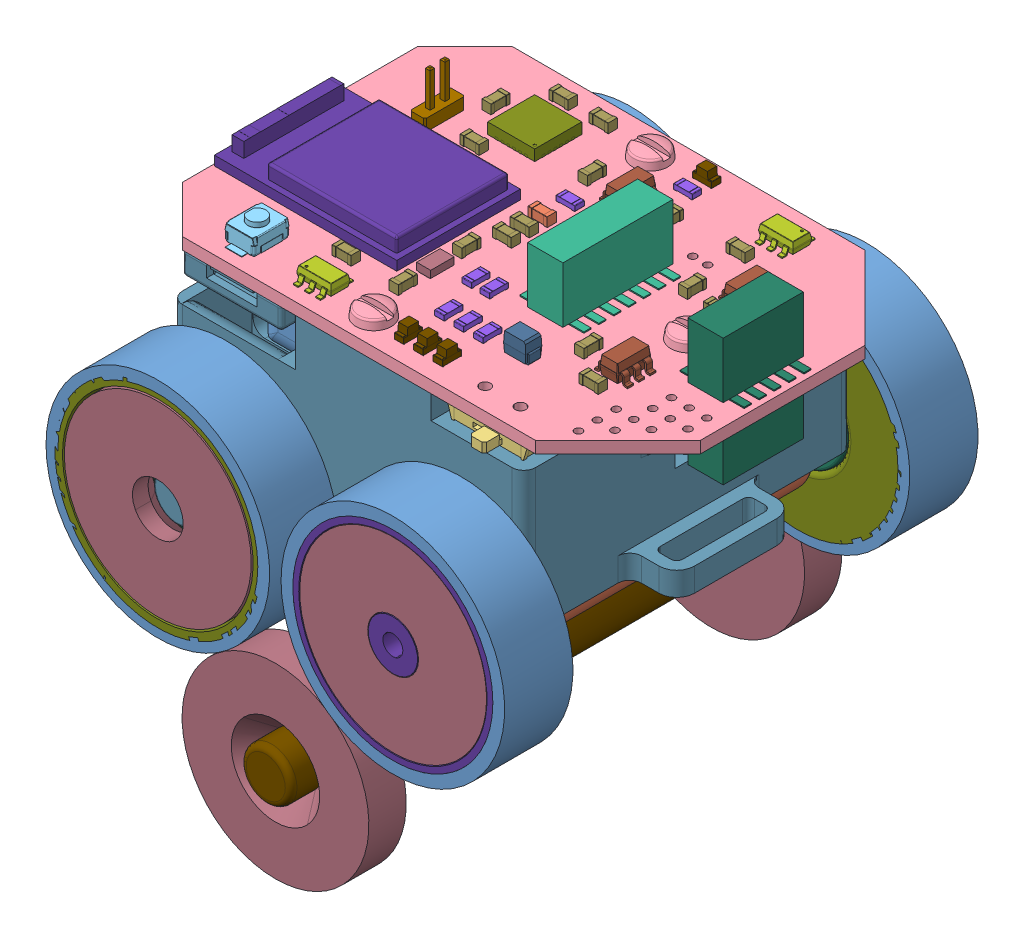
SolidWorks assembly AstroAnt, configuration Default. Lengths in mm.
Overall size (43.74 45.41 41.85).
158 component instances, 38 part files, 43 mates.
Components (placement in the parent):
- LiPo_360mAh-1: LiPo_360mAh [Default] at (6.8166 4.9998 44.2756) size (25 7 18)
- PA2-50-1: PA2-50 [Default] at (8.0673 -18.301 41.8029) x (0 0 1) z (0.952879 0.303349 0) size (29.1 8 8)
- PA2-50-2: PA2-50 [Default] at (-4.1563 19.5334 49.6029) x (0 0 -1) z (0.755989 -0.654584 0) size (29.1 8 8)
- 92120A150_Brass Heat-Set Inserts for Plastic-1: 92120A150_Brass Heat-Set Inserts for Plastic [92120A150] at (19.9543 12.4998 45.7029) size (2.56 3.33 2.56)
- 92120A150_Brass Heat-Set Inserts for Plastic-2: 92120A150_Brass Heat-Set Inserts for Plastic [92120A150] at (4.9543 12.4998 33.9529) size (2.56 3.33 2.56)
- 92120A150_Brass Heat-Set Inserts for Plastic-3: 92120A150_Brass Heat-Set Inserts for Plastic [92120A150] at (4.9543 12.4998 57.4529) size (2.56 3.33 2.56)
- 91460A005_METRIC CHEESE HEAD SLOTTED MACHINE SCREW-8: 91460A005_METRIC CHEESE HEAD SLOTTED MACHINE SCREW [91460A005] at (4.9543 14.9998 57.4529) x (1 0 0) z (0 1 0) size (3 3 7.1)
- 91460A005_METRIC CHEESE HEAD SLOTTED MACHINE SCREW-9: 91460A005_METRIC CHEESE HEAD SLOTTED MACHINE SCREW [91460A005] at (4.9543 14.9998 33.9529) x (1 0 0) z (0 1 0) size (3 3 7.1)
- 91460A005_METRIC CHEESE HEAD SLOTTED MACHINE SCREW-10: 91460A005_METRIC CHEESE HEAD SLOTTED MACHINE SCREW [91460A005] at (19.9543 14.9998 45.7029) x (1 0 0) z (0 1 0) size (3 3 7.1)
- 92120A150_Brass Heat-Set Inserts for Plastic-4: 92120A150_Brass Heat-Set Inserts for Plastic [92120A150] at (4.9543 1.4998 57.4529) x (-0.616962 0 -0.786993) z (0.786993 0 -0.616962) size (2.56 3.33 2.56)
- 92120A150_Brass Heat-Set Inserts for Plastic-5: 92120A150_Brass Heat-Set Inserts for Plastic [92120A150] at (4.9543 1.4998 33.9529) x (-0.616962 0 -0.786993) z (0.786993 0 -0.616962) size (2.56 3.33 2.56)
- 91460A005_METRIC CHEESE HEAD SLOTTED MACHINE SCREW-14: 91460A005_METRIC CHEESE HEAD SLOTTED MACHINE SCREW [91460A005] at (4.9543 -2.5002 57.4529) x (0.663599 0 0.748089) z (0 -1 0) size (3 3 7.1)
- 91460A005_METRIC CHEESE HEAD SLOTTED MACHINE SCREW-15: 91460A005_METRIC CHEESE HEAD SLOTTED MACHINE SCREW [91460A005] at (4.9543 -2.5002 33.9529) x (0.663599 0 0.748089) z (0 -1 0) size (3 3 7.1)
- mainboard_v1.step-1: mainboard_v1.step [Default] at (-103.0457 13.9998 235.7029) x (0 0 -1) z (0 1 0) size (29.41 41 10.8)
  - B3U-1000P.step-1: B3U-1000P.step [Default] at (178.95 -97.38 1.05) x (1 0 0) z (0 -1 0) size (4 1.75 2.5)
    - COMPOUND.step-1: COMPOUND.step [Default] at origin size (4 1.75 2.5)
  - 20021321-00014C1LF.step-1: 20021321-00014C1LF.step [Default] at (190 -115.5 1.05) size (9.35 5.45 4.85)
    - COMPOUND-0.step-1: COMPOUND-0.step [Default] at origin size (9.35 5.45 4.85)
  - MP6513GJ-Z.step-1: MP6513GJ-Z.step [Default] at (201.21 -120 1.05) x (-1 0 0) z (0 0 1) size (2.8 2.9 1)
    - COMPOUND-1.step-1: COMPOUND-1.step [Default] at origin size (2.8 2.9 1)
  - MP6513GJ-Z.step-2: MP6513GJ-Z.step [Default] at (178.51 -103.46 1.05) size (2.8 2.9 1)
    - COMPOUND-1.step-1: COMPOUND-1.step [Default] at origin size (2.8 2.9 1)
  - R_0603_1608Metric.step-1: R_0603_1608Metric.step [Default] at (195.55 -104.38 -0.05) x (1 0 0) z (0 0 -1) size (1.6 0.8 0.45)
    - SOLID.step-1: SOLID.step [Default] at origin size (1.6 0.8 0.45)
  - R_0603_1608Metric.step-2: R_0603_1608Metric.step [Default] at (192.6 -99.86 -0.05) x (0 1 0) z (0 0 -1) size (1.6 0.8 0.45)
    - SOLID.step-1: SOLID.step [Default] at origin size (1.6 0.8 0.45)
  - PinHeader_2x01_P1.27mm_Vertical.step-1: PinHeader_2x01_P1.27mm_Vertical.step [Default] at (194.96 -96.07 1.05) size (3.4 1.27 6.3)
    - SOLID-2.step-1: SOLID-2.step [Default] at origin size (3.4 1.27 6.3)
  - TAJP106K010RNJ.step-1: TAJP106K010RNJ.step [Default] at (196.22 -98.14 -0.05) x (-1 0 0) z (0 0 -1) size (2.05 1.4 1.7)
    - COMPOUND-3.step-1: COMPOUND-3.step [Default] at origin size (2.05 1.4 1.7)
  - TAJP106K010RNJ.step-2: TAJP106K010RNJ.step [Default] at (181.68 -117.23 1.05) x (0 1 0) z (0 0 1) size (2.05 1.4 1.7)
    - COMPOUND-3.step-1: COMPOUND-3.step [Default] at origin size (2.05 1.4 1.7)
  - SOT-23-5.step-1: SOT-23-5.step [Default] at (195.38 -122.78 1.05) x (0 1 0) z (0 0 1) size (2.8 2.9 1.55)
    - SOLID-4.step-1: SOLID-4.step [Default] at origin size (2.8 2.9 1.55)
  - C_0603_1608Metric.step-1: C_0603_1608Metric.step [Default] at (192.91 -122.55 1.05) x (0 -1 0) z (0 0 1) size (1.6 0.8 0.8)
    - SOLID-5.step-1: SOLID-5.step [Default] at origin size (1.6 0.8 0.8)
  - C_0603_1608Metric.step-2: C_0603_1608Metric.step [Default] at (193.57 -119.76 1.05) size (1.6 0.8 0.8)
    - SOLID-5.step-1: SOLID-5.step [Default] at origin size (1.6 0.8 0.8)
  - ECS-.327-12.5-12-TR.step-1: ECS-.327-12.5-12-TR.step [Default] at (184.31 -107.18 1.05) size (2 1.2 0.7)
    - COMPOUND-6.step-1: COMPOUND-6.step [Default] at origin size (2 1.2 0.7)
  - C_0603_1608Metric.step-3: C_0603_1608Metric.step [Default] at (197.67 -113.69 1.05) size (1.6 0.8 0.8)
    - SOLID-5.step-1: SOLID-5.step [Default] at origin size (1.6 0.8 0.8)
  - C_0603_1608Metric.step-4: C_0603_1608Metric.step [Default] at (197.64 -107.18 1.05) size (1.6 0.8 0.8)
    - SOLID-5.step-1: SOLID-5.step [Default] at origin size (1.6 0.8 0.8)
  - C_0603_1608Metric.step-5: C_0603_1608Metric.step [Default] at (190.96 -108.09 1.05) x (0 1 0) z (0 0 1) size (1.6 0.8 0.8)
    - SOLID-5.step-1: SOLID-5.step [Default] at origin size (1.6 0.8 0.8)
  - 1734592-6.step-1: 1734592-6.step [Default] at (203.79 -118 -1.05) x (0 -1 0) z (1 0 0) size (8.43 2.05 5.11)
    - SOLID-7.step-1: SOLID-7.step [Default] at origin size (8.43 2.05 5.11)
  - 1734592-6.step-2: 1734592-6.step [Default] at (176.19 -98 -1.05) x (0 1 0) z (-1 0 0) size (8.43 2.05 5.11)
    - SOLID-7.step-1: SOLID-7.step [Default] at origin size (8.43 2.05 5.11)
  - 20021321-00010C4LF.step-1: 20021321-00010C4LF.step [Default] at (190 -127.85 -0.05) x (1 0 0) z (0 0 -1) size (6.81 5.45 4.85)
    - COMPOUND-8.step-1: COMPOUND-8.step [Default] at origin size (6.81 5.45 4.85)
  - 20021321-00010C4LF.step-2: 20021321-00010C4LF.step [Default] at (190 -127.85 1.05) size (6.81 5.45 4.85)
    - COMPOUND-8.step-1: COMPOUND-8.step [Default] at origin size (6.81 5.45 4.85)
  - C_0603_1608Metric.step-6: C_0603_1608Metric.step [Default] at (181.31 -102.6 1.05) x (0 -1 0) z (0 0 1) size (1.6 0.8 0.8)
    - SOLID-5.step-1: SOLID-5.step [Default] at origin size (1.6 0.8 0.8)
  - C_0603_1608Metric.step-7: C_0603_1608Metric.step [Default] at (198.25 -119.14 1.05) x (0 -1 0) z (0 0 1) size (1.6 0.8 0.8)
    - SOLID-5.step-1: SOLID-5.step [Default] at origin size (1.6 0.8 0.8)
  - MPU6050.step-1: MPU6050.step [Default] at (198.43 -101.5 1.05) x (0 1 0) z (1 0 0) size (4 0.95 4)
    - COMPOUND-9.step-1: COMPOUND-9.step [Default] at origin size (4 0.95 4)
  - C_0603_1608Metric.step-8: C_0603_1608Metric.step [Default] at (194.9 -99.89 1.05) x (0 -1 0) z (0 0 1) size (1.6 0.8 0.8)
    - SOLID-5.step-1: SOLID-5.step [Default] at origin size (1.6 0.8 0.8)
  - C_0603_1608Metric.step-9: C_0603_1608Metric.step [Default] at (201.98 -100.38 1.05) x (0 -1 0) z (0 0 1) size (1.6 0.8 0.8)
    - SOLID-5.step-1: SOLID-5.step [Default] at origin size (1.6 0.8 0.8)
  - C_0603_1608Metric.step-10: C_0603_1608Metric.step [Default] at (201.98 -103.78 1.05) x (0 1 0) z (0 0 1) size (1.6 0.8 0.8)
    - SOLID-5.step-1: SOLID-5.step [Default] at origin size (1.6 0.8 0.8)
  - C_0603_1608Metric.step-11: C_0603_1608Metric.step [Default] at (198.81 -97.82 1.05) size (1.6 0.8 0.8)
    - SOLID-5.step-1: SOLID-5.step [Default] at origin size (1.6 0.8 0.8)
  - SOT-23-5.step-2: SOT-23-5.step [Default] at (184.86 -122.77 1.05) x (0 1 0) z (0 0 1) size (2.8 2.9 1.55)
    - SOLID-4.step-1: SOLID-4.step [Default] at origin size (2.8 2.9 1.55)
  - SOT-23-5.step-3: SOT-23-5.step [Default] at (197.58 -110.46 1.05) x (0 1 0) z (0 0 1) size (2.8 2.9 1.55)
    - SOLID-4.step-1: SOLID-4.step [Default] at origin size (2.8 2.9 1.55)
  - MDBT50Q-1MV2.step-1: MDBT50Q-1MV2.step [Default] at (187.3136 -98.605 1.0754) x (-1 0 0) z (0 1 0) size (10.5 2.06 15.5)
    - SOLID-10.step-1: SOLID-10.step [Default] at origin size (10.5 2.06 15.5)
  - C_0603_1608Metric.step-12: C_0603_1608Metric.step [Default] at (189.44 -108.09 1.05) x (0 1 0) z (0 0 1) size (1.6 0.8 0.8)
    - SOLID-5.step-1: SOLID-5.step [Default] at origin size (1.6 0.8 0.8)
  - C_0603_1608Metric.step-13: C_0603_1608Metric.step [Default] at (181.57 -107.18 1.05) x (-1 0 0) z (0 0 1) size (1.6 0.8 0.8)
    - SOLID-5.step-1: SOLID-5.step [Default] at origin size (1.6 0.8 0.8)
  - C_0603_1608Metric.step-14: C_0603_1608Metric.step [Default] at (186.97 -107.18 1.05) size (1.6 0.8 0.8)
    - SOLID-5.step-1: SOLID-5.step [Default] at origin size (1.6 0.8 0.8)
  - C_0603_1608Metric.step-15: C_0603_1608Metric.step [Default] at (184.77 -119.75 1.05) x (-1 0 0) z (0 0 1) size (1.6 0.8 0.8)
    - SOLID-5.step-1: SOLID-5.step [Default] at origin size (1.6 0.8 0.8)
  - C_0603_1608Metric.step-16: C_0603_1608Metric.step [Default] at (182.37 -122.54 1.05) x (0 -1 0) z (0 0 1) size (1.6 0.8 0.8)
    - SOLID-5.step-1: SOLID-5.step [Default] at origin size (1.6 0.8 0.8)
  - LED_0603_1608Metric.step-1: LED_0603_1608Metric.step [Default] at (178.19 -111.01 1.05) size (1.6 0.8 1.1)
    - SOLID-11.step-1: SOLID-11.step [Default] at origin size (1.6 0.8 1.1)
  - LED_0603_1608Metric.step-2: LED_0603_1608Metric.step [Default] at (178.19 -112.66 1.05) size (1.6 0.8 1.1)
    - SOLID-11.step-1: SOLID-11.step [Default] at origin size (1.6 0.8 1.1)
  - LED_0603_1608Metric.step-3: LED_0603_1608Metric.step [Default] at (178.19 -114.31 1.05) size (1.6 0.8 1.1)
    - SOLID-11.step-1: SOLID-11.step [Default] at origin size (1.6 0.8 1.1)
  - LED_0603_1608Metric.step-4: LED_0603_1608Metric.step [Default] at (202.34 -112.21 1.05) x (0 1 0) z (0 0 1) size (1.6 0.8 1.1)
    - SOLID-11.step-1: SOLID-11.step [Default] at origin size (1.6 0.8 1.1)
  - 473460001.step-1: 473460001.step [Default] at (201.68 -99.72 -1.25) x (0 -1 0) z (1 0 0) size (7.98 2.94 5.43)
    - COMPOUND-12.step-1: COMPOUND-12.step [Default] at origin size (7.98 2.94 5.43)
  - L_0603_1608Metric.step-1: L_0603_1608Metric.step [Default] at (192.48 -108.09 1.05) x (0 1 0) z (0 0 1) size (1.6 0.8 0.8)
    - SOLID-13.step-1: SOLID-13.step [Default] at origin size (1.6 0.8 0.8)
  - R_0603_1608Metric.step-3: R_0603_1608Metric.step [Default] at (185.18 -111.31 1.05) x (-1 0 0) z (0 0 1) size (1.6 0.8 0.45)
    - SOLID.step-1: SOLID.step [Default] at origin size (1.6 0.8 0.45)
  - R_0603_1608Metric.step-4: R_0603_1608Metric.step [Default] at (185.18 -109.77 1.05) size (1.6 0.8 0.45)
    - SOLID.step-1: SOLID.step [Default] at origin size (1.6 0.8 0.45)
  - R_0603_1608Metric.step-5: R_0603_1608Metric.step [Default] at (181.62 -111.01 1.05) size (1.6 0.8 0.45)
    - SOLID.step-1: SOLID.step [Default] at origin size (1.6 0.8 0.45)
  - R_0603_1608Metric.step-6: R_0603_1608Metric.step [Default] at (181.62 -112.66 1.05) size (1.6 0.8 0.45)
    - SOLID.step-1: SOLID.step [Default] at origin size (1.6 0.8 0.45)
  - R_0603_1608Metric.step-7: R_0603_1608Metric.step [Default] at (181.62 -114.31 1.05) x (-1 0 0) z (0 0 1) size (1.6 0.8 0.45)
    - SOLID.step-1: SOLID.step [Default] at origin size (1.6 0.8 0.45)
  - R_0603_1608Metric.step-8: R_0603_1608Metric.step [Default] at (194.84 -108.1 1.05) x (0 1 0) z (0 0 1) size (1.6 0.8 0.45)
    - SOLID.step-1: SOLID.step [Default] at origin size (1.6 0.8 0.45)
  - R_0603_1608Metric.step-9: R_0603_1608Metric.step [Default] at (200.69 -112.2325 1.05) x (0 1 0) z (0 0 1) size (1.6 0.8 0.45)
    - SOLID.step-1: SOLID.step [Default] at origin size (1.6 0.8 0.45)
  - R_0603_1608Metric.step-10: R_0603_1608Metric.step [Default] at (196.22 -101.51 -0.05) x (-1 0 0) z (0 0 -1) size (1.6 0.8 0.45)
    - SOLID.step-1: SOLID.step [Default] at origin size (1.6 0.8 0.45)
  - R_0603_1608Metric.step-11: R_0603_1608Metric.step [Default] at (196.22 -99.9725 -0.05) x (-1 0 0) z (0 0 -1) size (1.6 0.8 0.45)
    - SOLID.step-1: SOLID.step [Default] at origin size (1.6 0.8 0.45)
  - SW_SPDT_PCM12.step-1: SW_SPDT_PCM12.step [Default] at (178.18 -119.37 -0.05) x (0 1 0) z (0 0 -1) size (7.7 5 2)
    - SOLID-14.step-1: SOLID-14.step [Default] at origin size (7.7 5 2)
  - COMPOUND-15.step-1: COMPOUND-15.step [Default] at origin size (28 41 1)
- 91613A020_METRIC CHEESE HEAD SLOTTED MACHINE SCREW-1: 91613A020_METRIC CHEESE HEAD SLOTTED MACHINE SCREW [91613A020] at (1.2533 -0.5002 54.4029) x (1 0 0) z (0 1 0) size (3 3 5.08)
- 91613A020_METRIC CHEESE HEAD SLOTTED MACHINE SCREW-2: 91613A020_METRIC CHEESE HEAD SLOTTED MACHINE SCREW [91613A020] at (8.6533 -0.5002 54.4029) x (1 0 0) z (0 1 0) size (3 3 5.08)
- 91613A020_METRIC CHEESE HEAD SLOTTED MACHINE SCREW-3: 91613A020_METRIC CHEESE HEAD SLOTTED MACHINE SCREW [91613A020] at (1.2533 -0.5002 37.0029) x (1 0 0) z (0 1 0) size (3 3 5.08)
- IR_TEMP_V2.step-3: IR_TEMP_V2.step [Default] at (118.9553 -0.5002 109.7029) x (-1 0 0) z (0 1 0) size (10 20 4.8)
  - Board_Geoms_380f.step-1: Board_Geoms_380f.step [Default] at origin size (10 20 1.11)
    - Pcb_380f.step-1: Pcb_380f.step [Default] at origin size (10 20 1)
    - topTracks_380f.step-1: topTracks_380f.step [Default] at (0 0 0.01) size (9.62 17.53 0.05)
    - botTracks_380f.step-1: botTracks_380f.step [Default] at (0 0 -1.01) size (9.25 16.88 0.05)
  - Step_Models_380f.step-1: Step_Models_380f.step [Default] at origin size (9.46 10.17 4.8)
    - Top_380f.step-1: Top_380f.step [Default] at origin size (9.46 10.17 1.2)
      - IC1_PW14_613E6C6D.step-1: IC1_PW14_613E6C6D.step [Default] at (113.99 -59.48 0) x (-1 0 0) z (0 1 0) size (6.4 1.2 5)
      - C1_C_0402_1005Metric_613EDDF6.step-1: C1_C_0402_1005Metric_613EDDF6.step [Default] at (110.5 -64.26 0) x (-1 0 0) z (0 0 1) size (1 0.5 0.5)
      - C1_C_0402_1005Metric_613EDDF6.step-2: C1_C_0402_1005Metric_613EDDF6.step [Default] at (109.52 -61.07 0) x (0 -1 0) z (0 0 1) size (1 0.5 0.5)
      - C1_C_0402_1005Metric_613EDDF6.step-3: C1_C_0402_1005Metric_613EDDF6.step [Default] at (118.48 -60.86 0) x (0 -1 0) z (0 0 1) size (1 0.5 0.5)
      - C1_C_0402_1005Metric_613EDDF6.step-4: C1_C_0402_1005Metric_613EDDF6.step [Default] at (118.48 -58.59 0) x (0 -1 0) z (0 0 1) size (1 0.5 0.5)
      - C1_C_0402_1005Metric_613EDDF6.step-5: C1_C_0402_1005Metric_613EDDF6.step [Default] at (113.32 -66.9 0) size (1 0.5 0.5)
      - R1_R_0402_1005Metric_613EDE7A.step-1: R1_R_0402_1005Metric_613EDE7A.step [Default] at (110.98 -63.1 0) size (1 0.5 0.35)
      - R1_R_0402_1005Metric_613EDE7A.step-2: R1_R_0402_1005Metric_613EDE7A.step [Default] at (111.68 -66.3 0) x (0 1 0) z (0 0 1) size (1 0.5 0.35)
    - Bot_380f.step-1: Bot_380f.step [Default] at origin size (6.35 7.64 4.6)
      - U1_ZTP-135SR_613E6CD4.step-1: U1_ZTP-135SR_613E6CD4.step [Default] at (114 -64 -1) x (-1 0 0) z (0 -1 0) size (6.35 4.6 5.4)
      - C1_C_0402_1005Metric_613EDDF6.step-1: C1_C_0402_1005Metric_613EDDF6.step [Default] at (115.07 -59.56 -1) x (0 -1 0) z (0 0 -1) size (1 0.5 0.5)
      - R1_R_0402_1005Metric_613EDE7A.step-1: R1_R_0402_1005Metric_613EDE7A.step [Default] at (113.64 -59.58 -1) x (0 -1 0) z (0 0 -1) size (1 0.5 0.35)
- RA22CS-N.step-3: RA22CS-N.step [Default] at (-5.0457 -0.0002 27.1904) x (0.93329 0.359123 0) z (0.359123 -0.93329 0) size (15.88 3.17 15.88)
- Body_simple-1: Body_simple [Default] at (4.8007 -0.0002 38.7677) size (34 16 37)
- RA22CS-N.step-4: RA22CS-N.step [Default] at (14.9543 -0.0002 27.1904) x (0.986453 0.164042 0) z (0.164042 -0.986453 0) size (15.88 3.17 15.88)
- RA22CS-N.step-5: RA22CS-N.step [Default] at (4.9543 -14.2854 27.1904) x (0.988519 -0.1511 0) z (0.1511 0.988519 0) size (15.88 3.17 15.88)
- ball_bearing_5x11x4mm-1: ball_bearing_5x11x4mm [Default] at (-45.4624 -2.1758 28.9029) x (0.999925 -0.012245 0) z (0 0 1) size (8 8 2.5)
- wheel_holder_non_motor-1: wheel_holder_non_motor [Default] at (-70.2522 1.7638 25.6029) size (17.5 17.5 5.8)
- wheel_holder_non_motor-2: wheel_holder_non_motor [Default] at (-19.1131 -84.0559 65.8029) x (0.185441 0.982655 0) z (0 0 -1) size (17.5 17.5 5.8)
- ball_bearing_5x11x4mm-2: ball_bearing_5x11x4mm [Default] at (-30.2803 -54.9376 62.5029) x (0.373101 0.927791 0) z (0 0 -1) size (8 8 2.5)
- RA22CS-N.step-6: RA22CS-N.step [Default] at (-5.0457 -0.0002 64.2154) x (-0.469735 0.882807 0) z (-0.882807 -0.469735 0) size (15.88 3.17 15.88)
- RA22CS-N.step-7: RA22CS-N.step [Default] at (14.9543 -0.0002 64.2154) x (-0.206529 0.978441 0) z (-0.978441 -0.206529 0) size (15.88 3.17 15.88)
- wheel_motor-1: wheel_motor [Default] at (24.0366 1.7037 25.5779) size (17 17 5.8)
- wheel_motor-2: wheel_motor [Default] at (15.5431 29.126 65.8279) x (-0.038296 0.999266 0) z (0 0 -1) size (17 17 5.8)
- RA22CS-N.step-8: RA22CS-N.step [Default] at (4.9543 -14.2854 64.2154) x (-0.693236 -0.720711 0) z (-0.720711 0.693236 0) size (15.88 3.17 15.88)
- magnet_wheel_holder-1: magnet_wheel_holder [Default] at (28.927 -0.7064 28.7779) size (6 6 41.85)
- tire-1: tire [Default] at (38.167 -1.442 25.5779) size (19 19 5.8)
- tire-2: tire [Default] at (58.167 -1.442 25.6029) size (19 19 5.8)
- tire-3: tire [Default] at (38.167 -1.442 60.0029) size (19 19 5.8)
- tire-4: tire [Default] at (58.167 -1.442 60.0279) size (19 19 5.8)
- motor_holder-2: motor_holder [Default] at (-0.192 -4.5002 11.9282) size (20 4.13 28)
Mates (geometry in assembly coordinates):
- Coincident100: coincident anti-aligned: plane of mainboard_v1.step-1/COMPOUND-15.step-1 through (6.7692 13.9998 45.7029) normal (0 -1 0); plane of Body_simple-1 through (4.8007 13.9998 38.7677) normal (0 1 0)
- Concentric58: concentric anti-aligned: cylinder of PA2-50-2 through (-5.0457 -0.0002 33.4029) axis (0 0 1) radius 4; cylinder of Body_simple-1 through (-5.0457 -0.0002 57.7029) axis (0 0 -1) radius 4.1
- Concentric59: concentric aligned: cylinder of mainboard_v1.step-1/COMPOUND-15.step-1 through (19.9543 13.4998 45.7029) axis (0 1 0) radius 0.85; cylinder of Body_simple-1 through (19.9543 5.9998 45.7029) axis (0 1 0) radius 1.15
- Concentric60: concentric anti-aligned: cylinder of PA2-50-2 through (-5.0457 -0.0002 29.3029) axis (0 0 1) radius 1; cylinder of RA22CS-N.step-3 through (-5.0457 -0.0002 27.1904) axis (0 0 -1) radius 2.159
- Concentric63: concentric anti-aligned: cylinder of ball_bearing_5x11x4mm-1 through (14.9543 -0.0002 31.4029) axis (0 0 -1) radius 4; cylinder of wheel_holder_non_motor-1 through (14.9543 -0.0002 25.6029) axis (0 0 1) radius 4
- Concentric64: concentric aligned: cylinder of RA22CS-N.step-4 through (14.9543 -0.0002 28.7779) axis (0 0 -1) radius 7.9375; cylinder of wheel_holder_non_motor-1 through (14.9543 -0.0002 28.8029) axis (0 0 -1) radius 8.1
- Coincident103: coincident aligned: plane of RA22CS-N.step-4 through (14.9543 -0.0002 25.6029) normal (0 0 -1); plane of wheel_holder_non_motor-1 through (14.9543 -0.0002 25.6029) normal (0 0 -1)
- Concentric66: concentric anti-aligned: cylinder of Body_simple-1 through (14.9543 -0.0002 27.2029) axis (0 0 1) radius 2; cylinder of ball_bearing_5x11x4mm-1 through (14.9543 -0.0002 32.9029) axis (0 0 -1) radius 2
- Distance2: distance = 0.3 mm anti-aligned: plane of wheel_holder_non_motor-1 through (14.9543 -0.0002 31.4029) normal (0 0 1); plane of Body_simple-1 through (-10.0457 13.9998 31.7029) normal (0 0 -1)
- Coincident105: coincident aligned: plane of ball_bearing_5x11x4mm-1 through (14.9543 -0.0002 31.4029) normal (0 0 1); plane of wheel_holder_non_motor-1 through (14.9543 -0.0002 31.4029) normal (0 0 1)
- Distance3: distance = 0.3 mm anti-aligned: plane of wheel_holder_non_motor-2 through (-5.0457 -0.0002 60.0029) normal (0 0 -1); plane of Body_simple-1 through (-10.0457 13.9998 59.7029) normal (0 0 1)
- Concentric67: concentric aligned: cylinder of Body_simple-1 through (-5.0457 -0.0002 64.2029) axis (0 0 -1) radius 2; cylinder of wheel_holder_non_motor-2 through (-5.0457 -0.0002 65.8029) axis (0 0 -1) radius 4
- Coincident107: coincident aligned: plane of wheel_holder_non_motor-2 through (-5.0457 -0.0002 60.0029) normal (0 0 -1); plane of ball_bearing_5x11x4mm-2 through (-5.0457 -0.0002 60.0029) normal (0 0 -1)
- Concentric68: concentric anti-aligned: cylinder of Body_simple-1 through (-5.0457 -0.0002 64.2029) axis (0 0 -1) radius 2; cylinder of ball_bearing_5x11x4mm-2 through (-5.0457 -0.0002 58.5029) axis (0 0 1) radius 2
- Concentric69: concentric anti-aligned: cylinder of Body_simple-1 through (-5.0457 -0.0002 64.2029) axis (0 0 -1) radius 2; cylinder of RA22CS-N.step-6 through (-5.0457 -0.0002 64.2154) axis (0 0 1) radius 2.159
- Coincident108: coincident aligned: plane of wheel_holder_non_motor-2 through (-5.0457 -0.0002 65.8029) normal (0 0 1); plane of RA22CS-N.step-6 through (-5.0457 -0.0002 65.8029) normal (0 0 1)
- Coincident109: coincident aligned: plane of RA22CS-N.step-3 through (-5.0457 -0.0002 25.6029) normal (0 0 -1); plane of RA22CS-N.step-4 through (14.9543 -0.0002 25.6029) normal (0 0 -1)
- Concentric70: concentric anti-aligned: cylinder of PA2-50-2 through (-5.0457 -0.0002 29.3029) axis (0 0 1) radius 1; cylinder of RA22CS-N.step-3 through (-5.0457 -0.0002 27.1904) axis (0 0 -1) radius 2.159
- Concentric71: concentric anti-aligned: cylinder of PA2-50-1 through (14.9543 -0.0002 62.1029) axis (0 0 -1) radius 1; cylinder of RA22CS-N.step-7 through (14.9543 -0.0002 64.2154) axis (0 0 1) radius 2.159
- Concentric72: concentric anti-aligned: cylinder of PA2-50-1 through (14.9543 -0.0002 62.1029) axis (0 0 -1) radius 1; circle of RA22CS-N.step-7
- Coincident112: coincident aligned: plane of RA22CS-N.step-6 through (-5.0457 -0.0002 65.8029) normal (0 0 1); plane of RA22CS-N.step-7 through (14.9543 -0.0002 65.8029) normal (0 0 1)
- Coincident114: coincident anti-aligned: plane of RA22CS-N.step-3 through (-5.0457 -0.0002 28.7779) normal (0 0 1); plane of wheel_motor-1 through (-5.0457 -0.0002 28.7779) normal (0 0 -1)
- Concentric73: concentric aligned: cylinder of RA22CS-N.step-3 through (-5.0457 -0.0002 28.7779) axis (0 0 -1) radius 7.9375; cylinder of wheel_motor-1 through (-5.0457 -0.0002 28.7779) axis (0 0 -1) radius 8
- Concentric74: concentric aligned: cylinder of RA22CS-N.step-7 through (14.9543 -0.0002 62.6279) axis (0 0 1) radius 7.9375; cylinder of wheel_motor-2 through (14.9543 -0.0002 62.6279) axis (0 0 1) radius 8
- Coincident115: coincident anti-aligned: plane of RA22CS-N.step-7 through (14.9543 -0.0002 62.6279) normal (0 0 -1); plane of wheel_motor-2 through (14.9543 -0.0002 62.6279) normal (0 0 1)
- Coincident116: coincident aligned: plane of RA22CS-N.step-6 through (-5.0457 -0.0002 65.8029) normal (0 0 1); plane of RA22CS-N.step-7 through (14.9543 -0.0002 65.8029) normal (0 0 1)
- Coincident119: coincident aligned: plane of RA22CS-N.step-3 through (-5.0457 -0.0002 25.6029) normal (0 0 -1); plane of RA22CS-N.step-5 through (4.9543 -14.2854 25.6029) normal (0 0 -1)
- Concentric80: concentric anti-aligned: cylinder of RA22CS-N.step-5 through (4.9543 -14.2854 25.6029) axis (0 0 1) radius 7.9375; cylinder of RA22CS-N.step-8 through (4.9543 -14.2854 65.8029) axis (0 0 -1) radius 7.9375
- Coincident121: coincident aligned: plane of RA22CS-N.step-7 through (14.9543 -0.0002 65.8029) normal (0 0 1); plane of RA22CS-N.step-8 through (4.9543 -14.2854 65.8029) normal (0 0 1)
- Concentric82: concentric aligned: cylinder of RA22CS-N.step-5 through (4.9543 -14.2854 27.1904) axis (0 0 1) radius 2.159; cylinder of magnet_wheel_holder-1 through (4.9543 -14.2854 24.7779) axis (0 0 1) radius 2.16
- Coincident122: coincident anti-aligned: plane of RA22CS-N.step-8 through (4.9543 -14.2854 62.6279) normal (0 0 -1); plane of magnet_wheel_holder-1 through (4.9543 -14.2854 62.6279) normal (0 0 1)
- Concentric83: concentric anti-aligned: cylinder of wheel_motor-1 through (-5.0457 -0.0002 31.3779) axis (0 0 -1) radius 8.5; cylinder of tire-1 through (-5.0457 -0.0002 25.5779) axis (0 0 1) radius 8.5
- Coincident123: coincident aligned: plane of wheel_motor-1 through (-5.0457 -0.0002 25.5779) normal (0 0 -1); plane of tire-1 through (-5.0457 -0.0002 25.5779) normal (0 0 -1)
- Concentric84: concentric anti-aligned: cylinder of wheel_holder_non_motor-1 through (14.9543 -0.0002 31.4029) axis (0 0 -1) radius 8.75; cylinder of tire-2 through (14.9543 -0.0002 25.6029) axis (0 0 1) radius 8.5
- Coincident124: coincident aligned: plane of wheel_holder_non_motor-1 through (14.9543 -0.0002 25.6029) normal (0 0 -1); plane of tire-2 through (14.9543 -0.0002 25.6029) normal (0 0 -1)
- Coincident125: coincident aligned: plane of wheel_motor-2 through (14.9543 -0.0002 65.8279) normal (0 0 1); plane of tire-4 through (14.9543 -0.0002 65.8279) normal (0 0 1)
- Concentric85: concentric aligned: cylinder of wheel_motor-2 through (14.9543 -0.0002 60.0279) axis (0 0 1) radius 8.5; cylinder of tire-4 through (14.9543 -0.0002 60.0279) axis (0 0 1) radius 8.5
- Coincident126: coincident aligned: plane of wheel_holder_non_motor-2 through (-5.0457 -0.0002 65.8029) normal (0 0 1); plane of tire-3 through (-5.0457 -0.0002 65.8029) normal (0 0 1)
- Concentric86: concentric aligned: cylinder of wheel_holder_non_motor-2 through (-5.0457 -0.0002 60.0029) axis (0 0 1) radius 8.75; cylinder of tire-3 through (-5.0457 -0.0002 60.0029) axis (0 0 1) radius 8.5
- Concentric94: concentric anti-aligned: cylinder of IR_TEMP_V2.step-3/Step_Models_380f.step-1/Bot_380f.step-1/U1_ZTP-135SR_613E6CD4.step-1 through (4.9553 -4.1002 45.7029) axis (0 1 0) radius 2.35; cylinder of motor_holder-2 through (4.9553 -0.5002 45.7029) axis (0 -1 0) radius 2.5
- Coincident128: coincident anti-aligned: plane of IR_TEMP_V2.step-3/Board_Geoms_380f.step-1/Pcb_380f.step-1 through (4.9553 -1.5002 45.7029) normal (0 -1 0); plane of motor_holder-2 through (-0.192 -1.5002 11.9282) normal (0 1 0)
- Tangent5: tangent anti-aligned: cylinder of RA22CS-N.step-5 through (4.9543 -14.2854 25.6029) axis (0 0 1) radius 7.9375; cylinder of tire-2 through (14.9543 -0.0002 31.4029) axis (0 0 -1) radius 9.5
- Tangent6: tangent anti-aligned: cylinder of RA22CS-N.step-5 through (4.9543 -14.2854 25.6029) axis (0 0 1) radius 7.9375; cylinder of tire-1 through (-5.0457 -0.0002 31.3779) axis (0 0 -1) radius 9.5
